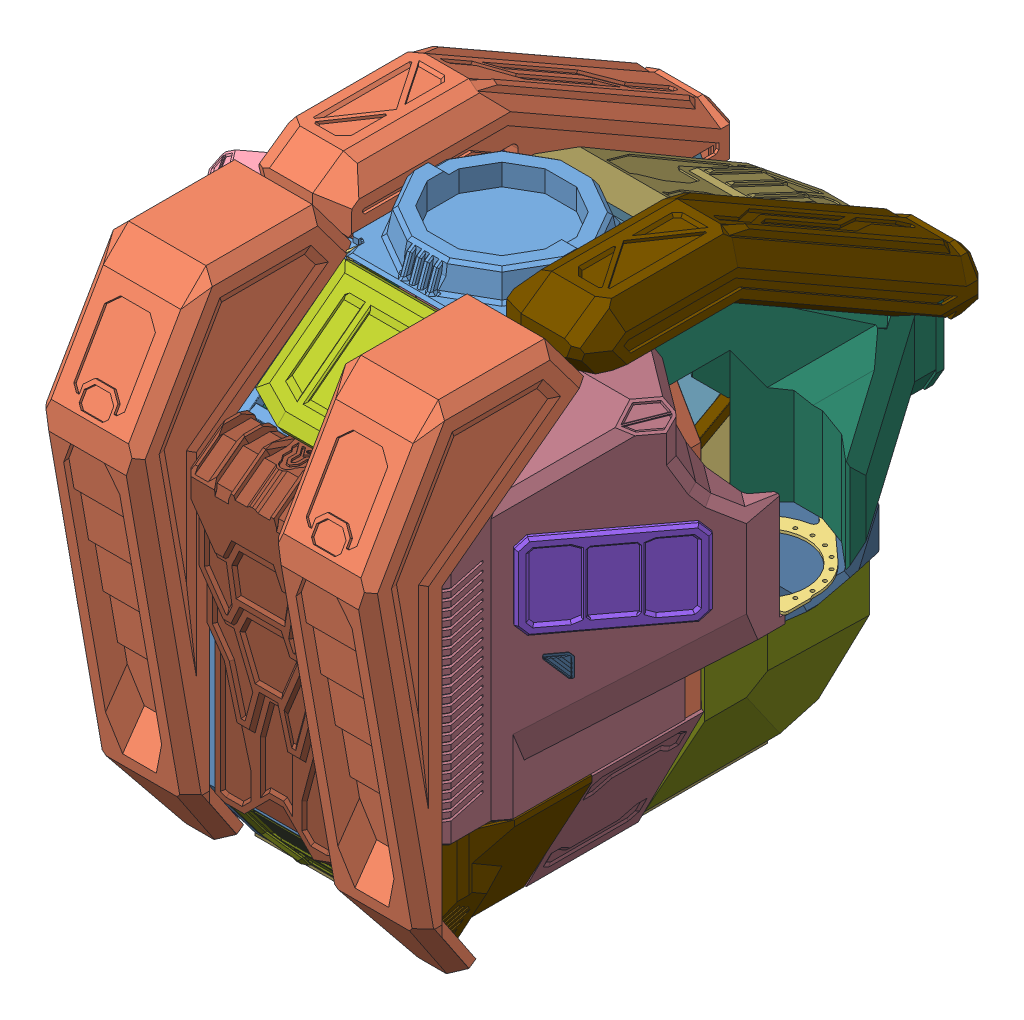
SolidWorks assembly Assemblage1_cockpit_v2, configuration Défaut. Lengths in mm. (continued)
Mates (geometry in assembly coordinates): (continued)
- Coaxiale6: concentric anti-aligned: cylinder of axeO20.25_700-1 through (100 1702.1061 -146.8375) axis (-1 0 0) radius 10; cylinder of Capot-1/Capot1-1 through (-490 1702.1061 -146.8375) axis (1 0 0) radius 10
- Distance5: distance = 10 mm anti-aligned: plane of Capot-1/Capot1-1 through (-490 1702.1061 -146.8375) normal (-1 0 0); plane of cockpit_segmentLAT_0-2 through (-500 0 0) normal (1 0 0)
- Coïncidente146: coincident anti-aligned: plane of bras_fixation_1-2 through (-1040 990 -47.0887) normal (0 -1 0); plane of deco_torse2LEFT-1 through (-931.6884 990 -630) normal (0 1 0)
- Coïncidente147: coincident anti-aligned: plane of cockpit_segmentLAT_0-2 through (-500 0 -740) normal (0 0 -1); plane of deco_torse2LEFT-1 through (-173.0822 150 -740) normal (0 0 1)
- Coïncidente148: coincident anti-aligned: plane of cockpit_segmentLAT_0-1 through (80 0 -740) normal (0 0 -1); plane of deco_torse2RIGHT-1 through (336.2329 150 -740) normal (0 0 1)
- Coïncidente149: coincident anti-aligned: plane of bras_fixation_1-1 through (540 990 -47.0887) normal (0 -1 0); plane of deco_torse2RIGHT-1 through (431.6884 990 -630) normal (0 1 0)
- Coïncidente150: coincident anti-aligned: plane of cockpit_segment_40x40_0-3 through (338 1000 -10) normal (0.942847 0 -0.333225); plane of deco_torse2RIGHT-1 through (336.2329 1000 -15) normal (-0.942847 0 0.333225)
- Coïncidente152: coincident anti-aligned: plane of cockpit_segment_40x40_0-4 through (-838 960 -10) normal (-0.942847 0 -0.333225); plane of deco_torse2LEFT-1 through (-836.2329 1000 -15) normal (0.942847 0 0.333225)
- Coïncidente153: coincident anti-aligned: plane of bras_fixation_1-1 through (540 1000 -47.0887) normal (0 1 0); plane of deco_torse1-1 through (277.9178 1000 -180) normal (0 -1 0)
- Coïncidente156: coincident anti-aligned: plane of cockpit_segmentLAT_0-1 through (80 0 -740) normal (0 0 -1); plane of deco_torse1-1 through (277.9178 1000 -740) normal (0 0 1)
- Coïncidente157: coincident anti-aligned: plane of cockpit_segment_40x40_0-1 through (338 1323.2129 -10) normal (0.942847 0 -0.333225); plane of deco_torse1-1 through (277.9178 1350 -180) normal (-0.942847 0 0.333225)
- Coïncidente166: coincident anti-aligned: plane of cockpit_segmentFACE_0-2 through (-593.1411 1740 413.3333) normal (0 1 0); plane of deco_headcollar-1 through (-540 1740 423.19) normal (0 -1 0)
- Coïncidente171: coincident anti-aligned: plane of cockpit_segmentLAT_0-1 through (80 1312 984) normal (0 0.8 0.6); plane of deco_torse4_back-1/deco_torse4_back-1 through (370 1630 560) normal (0 -0.8 -0.6)
- Coïncidente172: coincident anti-aligned: plane of cockpit_segmentLAT_0-2 through (-500 1312 984) normal (0 0.8 0.6); plane of deco_torse4_back-2/deco_torse4_back-1 through (-500 1630 560) normal (0 -0.8 -0.6)
- Coïncidente174: coincident anti-aligned: plane of cockpit_segmentLAT_0-1 through (80 0 960) normal (0 0 1); plane of deco_torse4_back-1/deco_torse4_back-1 through (370 250 960) normal (0 0 -1)
- Coïncidente175: coincident anti-aligned: plane of cockpit_segmentLAT_0-2 through (-500 0 960) normal (0 0 1); plane of deco_torse4_back-2/deco_torse4_back-1 through (-500 250 960) normal (0 0 -1)
- Coïncidente176: coincident aligned: plane of cockpit_segmentLAT_0-1 through (0 0 0) normal (-1 0 0); plane of attache_porte2-2 through (0 1717.0991 489.9076) normal (-1 0 0)
- Coïncidente177: coincident anti-aligned: plane of cockpit_segmentLAT_0-1 through (80 1312 984) normal (0 0.8 0.6); plane of attache_porte2-2 through (10 1737 417.3333) normal (0 -0.8 -0.6)
- Coïncidente180: coincident anti-aligned: plane of cockpit_segmentLAT_0-2 through (-500 1312 984) normal (0 0.8 0.6); plane of attache_porte2-4 through (-500 1737 417.3333) normal (0 -0.8 -0.6)
- Coïncidente181: coincident aligned: plane of cockpit_segmentLAT_0-2 through (-500 0 0) normal (1 0 0); plane of attache_porte2-4 through (-500 1717.0991 489.9076) normal (1 0 0)
- Coaxiale7: concentric aligned: cylinder of attache_porte2-2 through (10 1717.0991 489.9076) axis (-1 0 0) radius 23.5; cylinder of attache_porte2-4 through (-500 1717.0991 489.9076) axis (-1 0 0) radius 23.5
- Coïncidente182: coincident anti-aligned: plane of cockpit_segment_40x40_2_back-2 through (-840 1310.6802 413.3333) normal (-0.902861 0 0.429934); plane of deco_torse5_back-1 through (-674.9206 450 760) normal (0.902861 0 -0.429934)
- Coïncidente186: coincident aligned: plane of cockpit_segmentLAT_0-2 through (-500 0 0) normal (1 0 0); plane of deco_torse4_back-2/deco_torse4_back-1 through (-500 250 960) normal (1 0 0)
- Coïncidente189: coincident anti-aligned: plane of deco_torse4_back-2/deco_torse4_back-1 through (-500 250 960) normal (0 0 -1); plane of deco_torse5_back-1 through (-824.9206 450 960) normal (0 0 1)
- Coïncidente191: coincident anti-aligned: plane of cockpit_segmentLAT_0-2 through (-500 0 -740) normal (0 0 -1); plane of deco_torse1_sym-1 through (-238.4658 1000 -740) normal (0 0 1)
- Coïncidente194: coincident aligned: plane of deco_torse1-1 through (277.9178 1000 -180) normal (0 -1 0); plane of deco_torse1_sym-1 through (-777.9178 1000 -180) normal (0 -1 0)
- Coïncidente195: coincident anti-aligned: plane of cockpit_segment_40x40_0-2 through (-838 1283.2129 -10) normal (-0.942847 0 -0.333225); plane of deco_torse1_sym-1 through (-777.9178 1350 -180) normal (0.942847 0 0.333225)
- Coïncidente197: coincident: plane of deco_headcollar-1 through (-540 1740 423.19) normal (0 -1 0); line of attache_porte2-4 through (-500 1740 413.3333) axis (-1 0 0)
- Coaxiale8: concentric anti-aligned: cylinder of attache_porte2-2 through (10 1717.0991 489.9076) axis (-1 0 0) radius 23.5; cylinder of axeO20_520-1 through (-510 1717.0991 489.9076) axis (1 0 0) radius 10
- Coïncidente198: coincident aligned: plane of attache_porte2-4 through (-510 1717.0991 489.9076) normal (-1 0 0); plane of axeO20_520-1 through (-510 1717.0991 489.9076) normal (-1 0 0)
- Coaxiale9: concentric anti-aligned: cylinder of axeO20_520-1 through (-510 1717.0991 489.9076) axis (1 0 0) radius 10; cylinder of écoutille1-1 through (-5 1717.0991 489.9076) axis (-1 0 0) radius 10
- Distance8: distance = 5 mm anti-aligned: plane of écoutille1-1 through (-495 1761.0064 498.4018) normal (-1 0 0); plane of cockpit_segmentLAT_0-2 through (-500 0 0) normal (1 0 0)
- Coïncidente200: coincident anti-aligned: plane of deco_torse5_back-1 through (-1147.1119 1368.7153 314.3167) normal (0 -1 0); plane of back_trap-1 through (-1155.1093 1368.7153 320.3201) normal (0 1 0)
- Coïncidente201: coincident anti-aligned: plane of deco_torse5_back-1 through (-1165.1221 1098.7153 290.3244) normal (0.600343 0 0.799743); plane of back_trap-1 through (-1173.1196 1098.7153 296.3278) normal (-0.600343 0 -0.799743)
- Coïncidente202: coincident anti-aligned: plane of deco_torse5_back-1 through (-1234.9206 450 214) normal (-0.799743 0 0.600343); plane of back_trap-1 through (-1173.1196 1068.7153 296.3278) normal (0.799743 0 -0.600343)
- Coïncidente203: coincident anti-aligned: plane of bras_fixation_1-2 through (-1040 990 -47.0887) normal (0 -1 0); plane of deco_torse6_airvent-1 through (-834.9206 990 -640.6226) normal (0 1 0)
- Coïncidente204: coincident aligned: plane of deco_torse5_back-1 through (-1234.9206 450 69) normal (-1 0 0); plane of deco_torse6_airvent-1 through (-1234.9206 958 -640.6226) normal (-1 0 0)
- Coïncidente205: coincident anti-aligned: plane of deco_torse5_back-1 through (-1234.9206 450 214) normal (-0.799743 0 0.600343); plane of airvent-1 through (-958.7971 986.7153 581.836) normal (0.799743 0 -0.600343)
- Coïncidente206: coincident anti-aligned: plane of deco_torse5_back-1 through (-945.997 968.7153 582.2305) normal (0.600343 0 0.799743); plane of airvent-1 through (-949.9957 909.7153 585.2322) normal (-0.600343 0 -0.799743)
- Coïncidente207: coincident anti-aligned: plane of deco_torse5_back-1 through (-939.9935 978.7153 590.2279) normal (0 -1 0); plane of airvent-1 through (-943.8039 978.7153 593.4805) normal (0 1 0)
- Coïncidente208: coincident anti-aligned: plane of cockpit_poutre40x80x500-6 through (-500 1328 960) normal (0 0 1); plane of deco_torse7_dos-1 through (-500 230 960) normal (0 0 -1)
- Coïncidente211: coincident anti-aligned: plane of deco_torse4_back-1/deco_torse4_back-1 through (0 250 960) normal (-1 0 0); plane of deco_torse7_dos-1 through (0 230 960) normal (1 0 0)
- Coïncidente212: coincident anti-aligned: plane of cockpit_segmentLAT_0-1 through (80 1312 984) normal (0 0.8 0.6); plane of deco_torse7_dos-1 through (-500 1330 960) normal (0 -0.8 -0.6)
- Coïncidente213: coincident anti-aligned: plane of cockpit_segmentLAT_0-1 through (80 -40 0) normal (0 -1 0); plane of plancher-1 through (-580 -40 740.5405) normal (0 1 0)
- Coïncidente214: coincident: plane of cockpit_segmentLAT_0-1 through (80 0 0) normal (1 0 0); line of plancher-1 through (80 -40 740.5405) axis (0 0 -1)
- Coïncidente216: coincident: line of cockpit_segmentLAT_0-1 through (78 -40 740.5405) axis (-1 0 0); plane of plancher-1 through (-580 -40 740.5405) normal (0 0 1)
- Coïncidente219: coincident anti-aligned: plane of cockpit_segmentFACE_0-1 through (-840 440.3702 69.3774) normal (-0.890435 -0.455111 0); plane of deco_torse8_lateralinferieur-1 through (-599.1619 -30.8347 -6.6667) normal (0.890435 0.455111 0)
- Coïncidente220: coincident aligned: plane of cockpit_segmentFACE_0-2 through (-250 0 413.3333) normal (0 0 1); plane of deco_torse8_lateralinferieur-1 through (-608.0663 -35.3858 413.3333) normal (0 0 1)
- Coïncidente221: coincident: plane of deco_torse5_back-1 through (-674.9206 450 214) normal (0 -1 0); line of deco_torse8_lateralinferieur-1 through (-844.9219 450 413.3333) axis (0 0 -1)
- Coïncidente224: coincident anti-aligned: plane of cockpit_segmentFACE_0-1 through (340 440.3702 69.3774) normal (0.890435 -0.455111 0); plane of deco_torse8_lateralinferieur-2 through (99.1619 -30.8347 413.3333) normal (-0.890435 0.455111 0)
- Coïncidente225: coincident aligned: plane of cockpit_segmentFACE_0-2 through (-250 0 413.3333) normal (0 0 1); plane of deco_torse8_lateralinferieur-2 through (108.0663 -35.3858 413.3333) normal (0 0 1)
- Coïncidente226: coincident aligned: plane of cockpit_segmentLAT_0-1 through (0 0 0) normal (-1 0 0); plane of attache_porte-5 through (0 32.3991 -638.0132) normal (-1 0 0)
- Coïncidente227: coincident anti-aligned: plane of cockpit_segmentLAT_0-1 through (80 -278.2843 -278.2843) normal (0 -0.707107 -0.707107); plane of attache_porte-5 through (10 -33.8763 -522.6923) normal (0 0.707107 0.707107)
- Coïncidente228: coincident anti-aligned: plane of cockpit_segmentLAT_0-2 through (-500 -278.2843 -278.2843) normal (0 -0.707107 -0.707107); plane of attache_porte-6 through (-500 -33.8763 -522.6923) normal (0 0.707107 0.707107)
- Coïncidente229: coincident aligned: plane of cockpit_segmentLAT_0-2 through (-500 0 0) normal (1 0 0); plane of attache_porte-6 through (-500 32.3991 -638.0132) normal (1 0 0)
- Coïncidente230: coincident aligned: line of attache_porte-5 through (10 -40 -516.5685) axis (-1 0 0); line of attache_porte-6 through (-500 -40 -516.5685) axis (-1 0 0)
- Coïncidente232: coincident: plane of plancher-1 through (-580 -40 740.5405) normal (0 1 0); line of attache_porte-5 through (10 -40 -516.5685) axis (-1 0 0)
- Coïncidente233: coincident aligned: plane of attache_porte-5 through (10 32.3991 -638.0132) normal (1 0 0); plane of axeO20_520-2 through (10 32.3991 -638.0132) normal (1 0 0)
- Coaxiale10: concentric anti-aligned: cylinder of attache_porte-6 through (-500 32.3991 -638.0132) axis (-1 0 0) radius 23.5; cylinder of axeO20_520-2 through (-510 32.3991 -638.0132) axis (1 0 0) radius 10
- Coïncidente237: coincident anti-aligned: plane of cockpit_segmentLAT_0-1 through (80 -59.667 129.9889) normal (0 0.417168 -0.90883); plane of internalpanel1_back-1 through (-580 1402.9178 801.3393) normal (0 -0.417168 0.90883)
- Coïncidente238: coincident aligned: plane of cockpit_segmentLAT_0-2 through (-580 0 0) normal (-1 0 0); plane of internalpanel1_back-1 through (-580 1407.0895 792.251) normal (-1 0 0)
- Coïncidente239: coincident aligned: line of cockpit_segmentLAT_0-2 through (-502 485 380) axis (-1 0 0); line of internalpanel1_back-1 through (80 485 380) axis (-1 0 0)
- Coïncidente240: coincident anti-aligned: plane of cockpit_segmentFACE_0-1 through (-800 1300 69.3774) normal (1 0 0); plane of internalpanel2_side-2 through (-800 450 413.3774) normal (-1 0 0)
- Coïncidente241: coincident anti-aligned: line of cockpit_segmentFACE_0-2 through (-800 1300 411.3333) axis (0 0 -1); line of internalpanel2_side-2 through (-800 1300 -10.6226) axis (0 0 1)
- Coïncidente242: coincident anti-aligned: plane of cockpit_segmentFACE_0-1 through (300 1300 69.3774) normal (-1 0 0); plane of internalpanel2_side-1 through (300 450 -10.6226) normal (1 0 0)
- Coïncidente243: coincident aligned: line of cockpit_segmentFACE_0-1 through (300 1300 67.3774) axis (0 0 -1); line of internalpanel2_side-1 through (300 1300 413.3774) axis (0 0 -1)
- Coïncidente244: coincident aligned: plane of cockpit_segmentFACE_0-1 through (-250 0 -10.6226) normal (0 0 -1); plane of internalpanel2_side-1 through (290 450 -10.6226) normal (0 0 -1)
- Coïncidente245: coincident aligned: plane of cockpit_segmentFACE_0-1 through (-250 0 -10.6226) normal (0 0 -1); plane of internalpanel2_side-2 through (-790 450 -10.6226) normal (0 0 -1)
- Coïncidente246: coincident anti-aligned: plane of cockpit_segmentFACE_0-2 through (-570 1700 413.3333) normal (0.866906 -0.498471 0); plane of internalpanel3_upside-1 through (-799.2967 1301.2231 413.3774) normal (-0.866906 0.498471 0)
- Coïncidente247: coincident anti-aligned: plane of cockpit_segmentFACE_0-1 through (70 1700 69.3774) normal (-0.866906 -0.498471 0); plane of internalpanel3_upside-2 through (299.2967 1301.2231 -10.6226) normal (0.866906 0.498471 0)
- Coïncidente248: coincident aligned: plane of cockpit_segmentFACE_0-1 through (-250 0 -10.6226) normal (0 0 -1); plane of internalpanel3_upside-2 through (290.6277 1296.2384 -10.6226) normal (0 0 -1)
- Coïncidente249: coincident aligned: plane of cockpit_segmentFACE_0-1 through (-250 0 -10.6226) normal (0 0 -1); plane of internalpanel3_upside-1 through (-790.6277 1296.2384 -10.6226) normal (0 0 -1)
- Coïncidente250: coincident anti-aligned: line of cockpit_segmentFACE_0-1 through (-570 1700 67.3774) axis (0 0 -1); line of internalpanel3_upside-1 through (-570 1700 -10.6226) axis (0 0 1)
- Coïncidente251: coincident aligned: line of cockpit_segmentFACE_0-2 through (70 1700 411.3333) axis (0 0 -1); line of internalpanel3_upside-2 through (70 1700 413.3774) axis (0 0 -1)
- Coïncidente252: coincident anti-aligned: plane of cockpit_segmentFACE_0-1 through (-800 450 69.3774) normal (0.890435 0.455111 0); plane of internalpanel4_downside-2 through (-570 0 413.3333) normal (-0.890435 -0.455111 0)
- Coïncidente253: coincident aligned: plane of cockpit_segmentFACE_0-2 through (-250 0 413.3333) normal (0 0 1); plane of internalpanel4_downside-2 through (-561.0957 4.5511 413.3333) normal (0 0 1)
- Coïncidente254: coincident anti-aligned: plane of cockpit_segmentFACE_0-1 through (300 450 69.3774) normal (-0.890435 0.455111 0); plane of internalpanel4_downside-1 through (70 0 -10.6226) normal (0.890435 -0.455111 0)
- Coïncidente255: coincident aligned: plane of cockpit_segmentFACE_0-1 through (-250 0 -10.6226) normal (0 0 -1); plane of internalpanel4_downside-1 through (61.0957 4.5511 -10.6226) normal (0 0 -1)
- Coïncidente256: coincident anti-aligned: line of cockpit_segmentFACE_0-1 through (70 0 67.3774) axis (0 0 -1); line of internalpanel4_downside-1 through (70 0 -10.6226) axis (0 0 1)
- Coïncidente257: coincident aligned: line of cockpit_segmentFACE_0-1 through (-570 0 67.3774) axis (0 0 -1); line of internalpanel4_downside-2 through (-570 0 413.3333) axis (0 0 -1)
- Coïncidente258: coincident anti-aligned: plane of cockpit_segmentLAT_0-1 through (80 0 380) normal (0 0 -1); plane of internalpanel5_downback-1 through (80 0 380) normal (0 0 1)
- Coïncidente259: coincident anti-aligned: plane of cockpit_segmentFACE_0-2 through (70 0 413.3333) normal (0 1 0); plane of internalpanel5_downback-1 through (80 0 370) normal (0 -1 0)
- Coïncidente260: coincident aligned: plane of cockpit_segmentLAT_0-1 through (80 0 0) normal (1 0 0); plane of internalpanel5_downback-1 through (80 0 370) normal (1 0 0)
- Coïncidente261: coincident aligned: line of cockpit_segmentLAT_0-2 through (-502 0 -500) axis (-1 0 0); line of internalpanel6_floor-1 through (80 0 -500) axis (-1 0 0)
- Coïncidente262: coincident aligned: plane of cockpit_segmentLAT_0-1 through (80 0 0) normal (1 0 0); plane of internalpanel6_floor-1 through (80 10 -500) normal (1 0 0)
- Coïncidente263: coincident anti-aligned: plane of cockpit_segmentLAT_0-1 through (80 0 0) normal (0 1 0); plane of internalpanel6_floor-1 through (80 0 -500) normal (0 -1 0)
- Distance10: distance = 110 mm anti-aligned: plane of sparco style race seat 1-1 through (-452.7692 280 260) normal (0 0 1); plane of internalpanel5_downback-1 through (80 0 370) normal (0 0 -1)
- Distance11: distance = 270 mm anti-aligned: plane of sparco style race seat 1-1 through (-33.6692 280 -76.55) normal (0 -1 0); plane of internalpanel6_floor-1 through (80 10 -500) normal (0 1 0)
- Coïncidente275: coincident anti-aligned: line of internalpanel2_side-1 through (300 1300 -10.6226) axis (0 -1 0); line of internalpanel7_frontLEFT-2 through (300 450 -10.6226) axis (0 1 0)
- Coïncidente277: coincident: line of internalpanel2_side-1 through (290 1300 -10.6226) axis (1 0 0); plane of internalpanel7_frontLEFT-2 through (4.4348 1300 -700) normal (0 1 0)
- Coïncidente278: coincident: plane of cockpit_segmentLAT_0-1 through (80 0 -700) normal (0 0 1); line of internalpanel7_frontLEFT-2 through (4.4348 1300 -700) axis (0 -1 0)
- Coïncidente279: coincident: line of internalpanel2_side-2 through (-790 1300 -10.6226) axis (-1 0 0); plane of internalpanel8_frontRIGHT-1 through (-1077.08 1300 686.3901) normal (0 1 0)
- Coïncidente280: coincident aligned: line of internalpanel2_side-2 through (-800 450 -10.6226) axis (0 1 0); line of internalpanel8_frontRIGHT-1 through (-800 450 -10.6226) axis (0 1 0)
- Coïncidente282: coincident: plane of cockpit_segmentLAT_0-2 through (-500 0 -700) normal (0 0 1); line of internalpanel8_frontRIGHT-1 through (-504.4348 1300 -700) axis (0 -1 0)
- Coïncidente283: coincident aligned: line of internalpanel3_upside-2 through (61.3309 1695.0153 -10.6226) axis (0.498471 -0.866906 0); line of internalpanel9_frontLup-1 through (59.5239 1698.158 -10.6226) axis (0.498471 -0.866906 0)
- Coïncidente285: coincident: line of internalpanel7_frontLEFT-2 through (290.7574 1300 -6.8049) axis (-0.381763 0 -0.92426); point of internalpanel9_frontLup-1
- Coïncidente286: coincident anti-aligned: line of internalpanel3_upside-1 through (-790.6277 1296.2384 -10.6226) axis (0.498471 0.866906 0); line of internalpanel9_frontLup-2 through (-559.5239 1698.158 -10.6226) axis (-0.498471 -0.866906 0)
- Coïncidente287: coincident: line of internalpanel8_frontRIGHT-1 through (-504.4348 1300 -700) axis (-0.381763 0 0.92426); point of internalpanel9_frontLup-2
- Coïncidente291: coincident aligned: plane of internalpanel2_side-2 through (-790 1300 413.3774) normal (0 1 0); plane of internalpanel10_backsideLEFT-1 through (-790 1300 380) normal (0 1 0)
- Coïncidente296: coincident anti-aligned: line of internalpanel1_back-1 through (-580 485 380) axis (0 0.90883 0.417168); line of internalpanel10_backsideLEFT-1 through (-580 1300 754.0984) axis (0 -0.90883 -0.417168)
- Coïncidente297: coincident anti-aligned: line of internalpanel10_backsideLEFT-1 through (-580 527.1417 380) axis (-0.277211 0.960809 0); line of internalpanel10.5_backsideLEFT-1 through (-790 1254.9989 380) axis (0.277211 -0.960809 0)
- Coïncidente298: coincident anti-aligned: plane of internalpanel10_backsideLEFT-1 through (-790 485 380) normal (0 0 -1); plane of internalpanel10.5_backsideLEFT-1 through (-580 485 380) normal (0 0 1)
- Coïncidente299: coincident: point of internalpanel10_backsideLEFT-1; line of internalpanel10.5_backsideLEFT-1 through (-790 1254.9989 370) axis (0 0 1)
- Coïncidente300: coincident anti-aligned: line of internalpanel1_back-1 through (80 1407.0895 792.251) axis (0 -0.90883 -0.417168); line of internalpanel10_backsideRIGHT-1 through (80 527.1417 388.3406) axis (0 0.90883 0.417168)
- Coïncidente301: coincident aligned: plane of internalpanel10_backsideLEFT-1 through (-790 1300 380) normal (0 1 0); plane of internalpanel10_backsideRIGHT-1 through (290 1300 388.3406) normal (0 1 0)
- Coïncidente303: coincident anti-aligned: plane of internalpanel10_backsideRIGHT-1 through (290 485 388.3406) normal (0 0 -1); plane of internalpanel10.5_backsideRIGHT-1 through (80 485 388.3406) normal (0 0 1)
- Coïncidente304: coincident: point of internalpanel10_backsideRIGHT-1; line of internalpanel10.5_backsideRIGHT-1 through (290 1254.9989 378.3406) axis (0 0 1)
- Parallèle7: parallel anti-aligned: plane of cockpit_segmentLAT_0-1 through (80 0 0) normal (1 0 0); plane of internalpanel10.5_backsideRIGHT-1 through (80 35 388.3406) normal (-1 0 0)
- Coïncidente307: coincident anti-aligned: plane of cockpit_segment_40x40_1_soutien_bras-1 through (-840 990 -10.6226) normal (0 0 -1); plane of deco_torse6_airvent-1 through (-834.9206 990 -10.6226) normal (0 0 1)
- Coïncidente308: coincident anti-aligned: plane of cockpit_segment_40x40_1_soutien_bras-2 through (340 990 -10.6226) normal (0 0 -1); plane of deco_torse6_airventRIGHT-1 through (334.9136 990 -10.6226) normal (0 0 1)
- Coïncidente309: coincident anti-aligned: plane of bras_fixation_1-1 through (540 990 -47.0887) normal (0 -1 0); plane of deco_torse6_airventRIGHT-1 through (334.9136 990 -640.6226) normal (0 1 0)
- Coïncidente310: coincident anti-aligned: plane of deco_torse2RIGHT-1 through (431.6884 1000 -15) normal (0.942847 0 -0.333225); plane of deco_torse6_airventRIGHT-1 through (348.4136 608 -250.6226) normal (-0.942847 0 0.333225)
- Coïncidente312: coincident anti-aligned: plane of cockpit_segmentLAT_0-2 through (-580 0 0) normal (-1 0 0); plane of internalpanel11_backsideUPLEFT-1 through (-580 1310.6802 413.3774) normal (1 0 0)
- Coïncidente314: coincident anti-aligned: plane of internalpanel3_upside-1 through (-790.6277 1296.2384 413.3774) normal (0 0 1); plane of internalpanel11_backsideUPLEFT-1 through (-580 1610.6802 413.3774) normal (0 0 -1)
- Coïncidente318: coincident anti-aligned: plane of cockpit_segment_40x40_2_back-2 through (-580 1310.6802 413.3333) normal (0 1 0); plane of internalpanel11_backsideUPLEFT-1 through (-580 1310.6802 813.3774) normal (0 -1 0)
- Coïncidente319: coincident anti-aligned: plane of cockpit_segmentFACE_0-2 through (-250 0 413.3333) normal (0 0 1); plane of internalpanel11_backsideUPRIGHT-1 through (80 1612.1 413.3333) normal (0 0 -1)
- Coïncidente320: coincident anti-aligned: plane of cockpit_segmentLAT_0-1 through (80 0 0) normal (1 0 0); plane of internalpanel11_backsideUPRIGHT-1 through (80 1677.3174 413.3333) normal (-1 0 0)
- Coïncidente321: coincident anti-aligned: plane of cockpit_segmentLAT_0-1 through (80 1280 960) normal (0 -0.8 -0.6); plane of internalpanel11_backsideUPRIGHT-1 through (80 1690 413.3333) normal (0 0.8 0.6)
- Coïncidente322: coincident aligned: plane of deco_torse5_back-1 through (-674.9206 1740 214) normal (0 1 0); plane of deco_torse5_backRIGHT-1 through (174 1740 214) normal (0 1 0)
- Coïncidente323: coincident anti-aligned: plane of cockpit_segmentLAT_0-1 through (80 0 0) normal (1 0 0); plane of deco_torse5_backRIGHT-1 through (80 1000 214) normal (-1 0 0)
- Coïncidente324: coincident aligned: plane of deco_torse5_back-1 through (-824.9206 450 960) normal (0 0 1); plane of deco_torse5_backRIGHT-1 through (324 450 960) normal (0 0 1)
- Coïncidente325: coincident anti-aligned: plane of deco_torse5_backRIGHT-1 through (646.1912 1368.7153 314.3167) normal (0 -1 0); plane of back_trap-2 through (384.0343 1368.7153 680.2043) normal (0 1 0)
- Coïncidente326: coincident anti-aligned: plane of deco_torse5_backRIGHT-1 through (664.2015 1098.7153 290.3244) normal (-0.600343 0 0.799743); plane of back_trap-2 through (672.1989 1098.7153 296.3278) normal (0.600343 0 -0.799743)
- Coïncidente327: coincident anti-aligned: plane of deco_torse5_backRIGHT-1 through (734 450 214) normal (0.799743 0 0.600343); plane of back_trap-2 through (366.024 1068.7153 704.1966) normal (-0.799743 0 -0.600343)
- Coïncidente328: coincident anti-aligned: plane of deco_torse5_backRIGHT-1 through (439.0729 978.7153 590.2279) normal (0 -1 0); plane of airvent-2 through (407.6514 978.7153 640.4144) normal (0 1 0)
- Coïncidente329: coincident anti-aligned: plane of deco_torse5_backRIGHT-1 through (734 450 214) normal (0.799743 0 0.600343); plane of airvent-2 through (457.8765 986.7153 581.836) normal (-0.799743 0 -0.600343)
- Coïncidente330: coincident anti-aligned: plane of deco_torse5_backRIGHT-1 through (445.0763 968.7153 582.2305) normal (-0.600343 0 0.799743); plane of airvent-2 through (449.075 968.4016 585.2322) normal (0.600343 0 -0.799743)
- Coïncidente332: coincident aligned: plane of deco_torse1_sym-1 through (-777.9178 1350 -180) normal (0 1 0); plane of front_trapLEFT-1 through (-608.1918 1350 -960) normal (0 1 0)
- Coïncidente334: coincident aligned: line of deco_torse1_sym-1 through (-819.9178 1300 -910) axis (0 -1 0); line of front_trapLEFT-1 through (-819.9178 1300 -910) axis (0 -1 0)
- Coïncidente336: coincident aligned: plane of deco_torse1-1 through (277.9178 1350 -180) normal (0 1 0); plane of front_trapRIGHT-1 through (108.1918 1350 -960) normal (0 1 0)
- Coïncidente338: coincident aligned: line of deco_torse1-1 through (319.9178 1300 -910) axis (0 -1 0); line of front_trapRIGHT-1 through (319.9178 1300 -910) axis (0 -1 0)
- Coïncidente343: coincident: plane of cockpit_poutre40x80x500-5 through (0 250 922) normal (0 -1 0); line of deco_torse9_backbas-1 through (-110 250 958.9927) axis (-1 0 0)
- Parallèle9: parallel aligned: plane of cockpit_segmentLAT_0-1 through (80 -370.9057 490.1254) normal (0 -0.603443 0.797406); plane of deco_torse9_backbas-1 through (-500 -44.7272 729.6857) normal (0 -0.603443 0.797406)
- Coïncidente344: coincident anti-aligned: plane of cockpit_segmentLAT_0-1 through (0 0 0) normal (-1 0 0); plane of deco_torse9_backbas-1 through (0 -47.7444 733.6727) normal (1 0 0)
- Coïncidente345: coincident: line of deco_torse7_dos-1 through (-110 230 960) axis (1 0 0); plane of deco_torse9_backbas-1 through (-451.7567 -45.3016 973.865) normal (0 0.050299 0.998734)
- Coïncidente346: coincident: line of deco_torse8_lateralinferieur-2 through (344.9219 450 -6.6667) axis (0 0 1); plane of deco_torse5_backRIGHT-1 through (174 450 214) normal (0 -1 0)
- Coïncidente347: coincident anti-aligned: plane of cockpit_segmentLAT_0-2 through (-580 0 0) normal (-1 0 0); plane of deco_torse10_backbassideLEFT-1 through (-580 -40 963.3333) normal (1 0 0)
- Coïncidente348: coincident anti-aligned: plane of deco_torse5_back-1 through (-674.9206 450 214) normal (0 -1 0); plane of deco_torse10_backbassideLEFT-1 through (-855 450 963.3333) normal (0 1 0)
- Coïncidente349: coincident anti-aligned: plane of cockpit_segmentFACE_0-2 through (-250 0 413.3333) normal (0 0 1); plane of deco_torse10_backbassideLEFT-1 through (-855 -40 413.3333) normal (0 0 -1)
- Coïncidente350: coincident anti-aligned: plane of cockpit_segmentLAT_0-1 through (80 0 0) normal (1 0 0); plane of deco_torse10_backbassideRIGHT-1 through (80 -40 943.3333) normal (-1 0 0)
- Coïncidente351: coincident anti-aligned: plane of deco_torse5_backRIGHT-1 through (174 450 214) normal (0 -1 0); plane of deco_torse10_backbassideRIGHT-1 through (-195 450 963.3333) normal (0 1 0)
- Coïncidente352: coincident anti-aligned: plane of cockpit_segmentFACE_0-2 through (-250 0 413.3333) normal (0 0 1); plane of deco_torse10_backbassideRIGHT-1 through (-195 -40 413.3333) normal (0 0 -1)
- Coaxiale11: concentric anti-aligned: cylinder of axeO20_520-2 through (-510 32.3991 -638.0132) axis (1 0 0) radius 10; cylinder of écoutille2-1 through (0 32.3991 -638.0132) axis (-1 0 0) radius 10
- Coïncidente353: coincident anti-aligned: plane of attache_porte-5 through (0 32.3991 -638.0132) normal (-1 0 0); plane of écoutille2-1 through (0 549.3297 -926.0153) normal (1 0 0)
- Coïncidente358: coincident anti-aligned: plane of attache_porte-4 through (10 1702.1061 -146.8375) normal (1 0 0); plane of deco_headcollar-1 through (10 1760 -106.81) normal (-1 0 0)
- Coïncidente366: coincident anti-aligned: plane of deco_torse1-1 through (360 1350 -740) normal (0 0.868243 -0.496139); plane of deco_torse3_upRIGHT-1 through (390.1918 1340 -757.5) normal (0 -0.868243 0.496139)
- Coïncidente367: coincident anti-aligned: plane of deco_torse1_sym-1 through (-860 1350 -740) normal (0 0.868243 -0.496139); plane of deco_torse3_upLEFT-1 through (-190.1918 1340 -757.5) normal (0 -0.868243 0.496139)
- Coïncidente371: coincident anti-aligned: plane of front_trapLEFT-1 through (-508.1918 1176.7949 -960) normal (0.866025 0.5 0); plane of deco_torse3_upLEFT-1 through (-508.1918 1176.7949 -1026.7218) normal (-0.866025 -0.5 0)
- Coïncidente372: coincident anti-aligned: plane of deco_torse3_upRIGHT-1 through (8.1918 1176.7949 -1026.7218) normal (0.866025 -0.5 0); plane of front_trapRIGHT-1 through (8.1918 1176.7949 -960) normal (-0.866025 0.5 0)
- Coïncidente376: coincident anti-aligned: plane of cockpit_segmentLAT_0-2 through (-500 1740 0) normal (0 1 0); plane of deco_torse3_upLEFT-1 through (-190.1918 1740 642.5) normal (0 -1 0)
- Coïncidente377: coincident anti-aligned: plane of bras_fixation_1-2 through (-1040 990 -47.0887) normal (0 -1 0); plane of deco_torse5_back-1 through (-674.9206 990 214) normal (0 1 0)
- Coïncidente378: coincident anti-aligned: plane of cockpit_segmentLAT_0-2 through (-500 0 0) normal (1 0 0); plane of deco_torse7_dos-1 through (-500 230 960) normal (-1 0 0)
- Coïncidente379: coincident anti-aligned: plane of cockpit_segmentFACE_0-2 through (-250 0 333.3333) normal (0 0 -1); plane of attache_verin_cokpitepaul-2 through (-840 1200.6802 333.3333) normal (0 0 1)
- Coïncidente380: coincident anti-aligned: plane of cockpit_segmentFACE_0-2 through (-840 1310.6802 413.3333) normal (-1 0 0); plane of attache_verin_cokpitepaul-2 through (-840 1200.6802 333.3333) normal (1 0 0)
- Coïncidente381: coincident anti-aligned: plane of cockpit_segmentFACE_0-2 through (-250 0 333.3333) normal (0 0 -1); plane of attache_verin_cokpitepaul-1 through (-840 1270.6802 333.3333) normal (0 0 1)
- Coïncidente382: coincident anti-aligned: plane of cockpit_segmentFACE_0-2 through (-840 1310.6802 413.3333) normal (-1 0 0); plane of attache_verin_cokpitepaul-1 through (-840 1270.6802 333.3333) normal (1 0 0)
- Coïncidente383: coincident anti-aligned: plane of cockpit_segmentFACE_0-2 through (340 1310.6802 413.3333) normal (1 0 0); plane of attache_verin_cokpitepaul-3 through (340 1260.6802 333.3333) normal (-1 0 0)
- Coïncidente384: coincident anti-aligned: plane of cockpit_segmentFACE_0-2 through (-250 0 333.3333) normal (0 0 -1); plane of attache_verin_cokpitepaul-3 through (340 1260.6802 333.3333) normal (0 0 1)
- Coïncidente386: coincident anti-aligned: plane of cockpit_segmentFACE_0-2 through (-250 0 333.3333) normal (0 0 -1); plane of attache_verin_cokpitepaul-4 through (340 1200.6802 333.3333) normal (0 0 1)
- Coïncidente387: coincident anti-aligned: plane of cockpit_segmentFACE_0-2 through (340 1310.6802 413.3333) normal (1 0 0); plane of attache_verin_cokpitepaul-4 through (340 1200.6802 333.3333) normal (-1 0 0)
- Coïncidente389: coincident anti-aligned: plane of cockpit_poutre40x40x366-1 through (-838 1270.6802 333.3333) normal (0 -1 0); plane of attache_verin_cokpitepaul-1 through (-867.2236 1270.6802 306.1097) normal (0 1 0)
- Distance13: distance = 60 mm anti-aligned: plane of attache_verin_cokpitepaul-1 through (-867.2236 1260.6802 306.1097) normal (0 -1 0); plane of attache_verin_cokpitepaul-2 through (-867.2236 1200.6802 306.1097) normal (0 1 0)
- Coïncidente388: coincident anti-aligned: plane of cockpit_poutre40x40x366-3 through (302 1270.6802 333.3774) normal (0 -1 0); plane of attache_verin_cokpitepaul-3 through (367.2236 1270.6802 306.1097) normal (0 1 0)
- Distance16: distance = 60 mm anti-aligned: plane of attache_verin_cokpitepaul-4 through (367.2236 1200.6802 306.1097) normal (0 1 0); plane of attache_verin_cokpitepaul-3 through (367.2236 1260.6802 306.1097) normal (0 -1 0)
